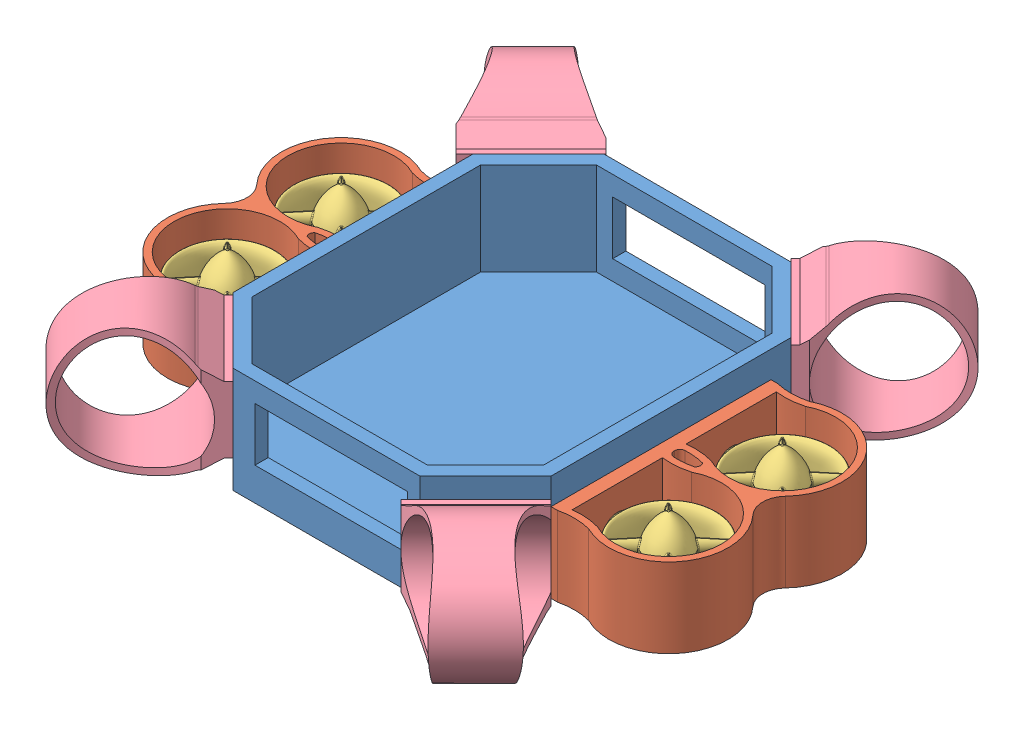
SolidWorks assembly FONKYTOWN, configuration Default. Lengths in mm.
Overall size (542.92 164.73 552.6).
13 component instances, 4 part files, 11 mates.
Components (placement in the parent):
- HexAPod-1: HexAPod [Default] at (133.0391 134.2869 240.6254) size (304.8 101.6 355.6)
- CR-A-0004b-VerticalMotorAssem-1: CR-A-0004b-VerticalMotorAssem [Default] at (-146.9254 393.2446 76.2323) x (1 0 0) z (0 -1 0) size (119.06 223.52 112.68)
  - CR-P-0005b-Frame-MotorMount Vertical-1: CR-P-0005b-Frame-MotorMount Vertical [Default] at (65.652 113.9901 182.7577) size (119.06 223.52 76.2)
  - CR-P-0003-T200-THRUSTER-R1-1: CR-P-0003-T200-THRUSTER-R1 [Default] at (65.8645 223.2101 226.1095) x (0 -1 0) z (0 0 1) size (96.71 97.53 112.68)
  - CR-P-0003-T200-THRUSTER-R1-2: CR-P-0003-T200-THRUSTER-R1 [Default] at (65.8645 113.9901 226.1095) x (0 -1 0) z (0 0 1) size (96.71 97.53 112.68)
- CR-A-0004b-VerticalMotorAssem-2: CR-A-0004b-VerticalMotorAssem [Default] at (413.0036 393.2446 418.7537) x (-1 0 0) z (0 -1 0) size (119.06 223.52 112.68)
  - CR-P-0005b-Frame-MotorMount Vertical-1: CR-P-0005b-Frame-MotorMount Vertical [Default] at (65.652 113.9901 182.7577) size (119.06 223.52 76.2)
  - CR-P-0003-T200-THRUSTER-R1-1: CR-P-0003-T200-THRUSTER-R1 [Default] at (65.8645 223.2101 226.1095) x (0 -1 0) z (0 0 1) size (96.71 97.53 112.68)
  - CR-P-0003-T200-THRUSTER-R1-2: CR-P-0003-T200-THRUSTER-R1 [Default] at (65.8645 113.9901 226.1095) x (0 -1 0) z (0 0 1) size (96.71 97.53 112.68)
- fonky-1: fonky [Default] at (-2.5934 204.1369 14.8065) x (-0.707107 0 0.707107) z (-0.707107 0 -0.707107) size (109.52 120.65 126.87)
- fonky-2: fonky [Default] at (338.5767 204.1369 84.7117) x (-0.707107 0 -0.707107) z (0.707107 0 -0.707107) size (109.52 120.65 126.87)
- fonky-3: fonky [Default] at (260.5577 184.7115 474.558) x (0.707107 0 -0.707107) z (0.707107 0 0.707107) size (109.52 120.65 126.87)
- fonky-4: fonky [Default] at (-74.9617 193.4476 394.0759) x (0.707107 0 0.707107) z (-0.707107 0 0.707107) size (109.52 120.65 126.87)
Mates (geometry in assembly coordinates):
- Coincident1: coincident anti-aligned: plane of HexAPod-1 through (-19.3609 235.8869 240.6254) normal (-1 0 0); plane of CR-A-0004b-VerticalMotorAssem-1/CR-P-0005b-Frame-MotorMount Vertical-1 through (-19.3609 210.4869 190.2224) normal (1 0 0)
- Coincident2: coincident aligned: plane of HexAPod-1 through (133.0391 134.2869 240.6254) normal (0 -1 0); plane of CR-A-0004b-VerticalMotorAssem-1/CR-P-0005b-Frame-MotorMount Vertical-1 through (-81.2734 134.2869 190.2224) normal (0 -1 0)
- Coincident3: coincident anti-aligned: plane of HexAPod-1 through (285.4391 235.8869 240.6254) normal (1 0 0); plane of CR-A-0004b-VerticalMotorAssem-2/CR-P-0005b-Frame-MotorMount Vertical-1 through (285.4391 210.4869 304.7636) normal (-1 0 0)
- Coincident4: coincident aligned: plane of HexAPod-1 through (133.0391 134.2869 240.6254) normal (0 -1 0); plane of CR-A-0004b-VerticalMotorAssem-2/CR-P-0005b-Frame-MotorMount Vertical-1 through (347.3516 134.2869 304.7636) normal (0 -1 0)
- Coincident5: coincident: line of HexAPod-1 through (285.4391 235.8869 355.5636) axis (0 -1 0); plane of CR-A-0004b-VerticalMotorAssem-2/CR-P-0005b-Frame-MotorMount Vertical-1 through (285.4391 210.4869 355.5636) normal (0 0 1)
- Coincident7: coincident: plane of HexAPod-1 through (-0.63 235.8869 106.9563) normal (-0.707107 0 -0.707107); plane of fonky-1 through (-24.8681 180.542 131.1943) normal (0.707107 0 0.707107)
- Coincident9: coincident: plane of HexAPod-1 through (266.7082 235.8869 106.9563) normal (0.707107 0 -0.707107); plane of fonky-2 through (219.5252 190.2726 59.7733) normal (-0.707107 0 0.707107)
- Coincident10: coincident anti-aligned: plane of HexAPod-1 through (266.7082 235.8869 374.2945) normal (0.707107 0 0.707107); plane of fonky-3 through (285.3432 184.7115 355.6595) normal (-0.707107 0 -0.707107)
- Coincident11: coincident anti-aligned: plane of HexAPod-1 through (-0.63 235.8869 374.2945) normal (-0.707107 0 0.707107); plane of fonky-4 through (43.9369 193.4476 418.8614) normal (0.707107 0 -0.707107)
- Coincident12: coincident aligned: plane of HexAPod-1 through (133.0391 235.8869 240.6254) normal (0 1 0); plane of fonky-1 through (-74.4354 235.8869 86.6485) normal (0 1 0)
- Coincident13: coincident aligned: plane of HexAPod-1 through (133.0391 235.8869 240.6254) normal (0 1 0); plane of fonky-2 through (266.7347 235.8869 12.8697) normal (0 1 0)
